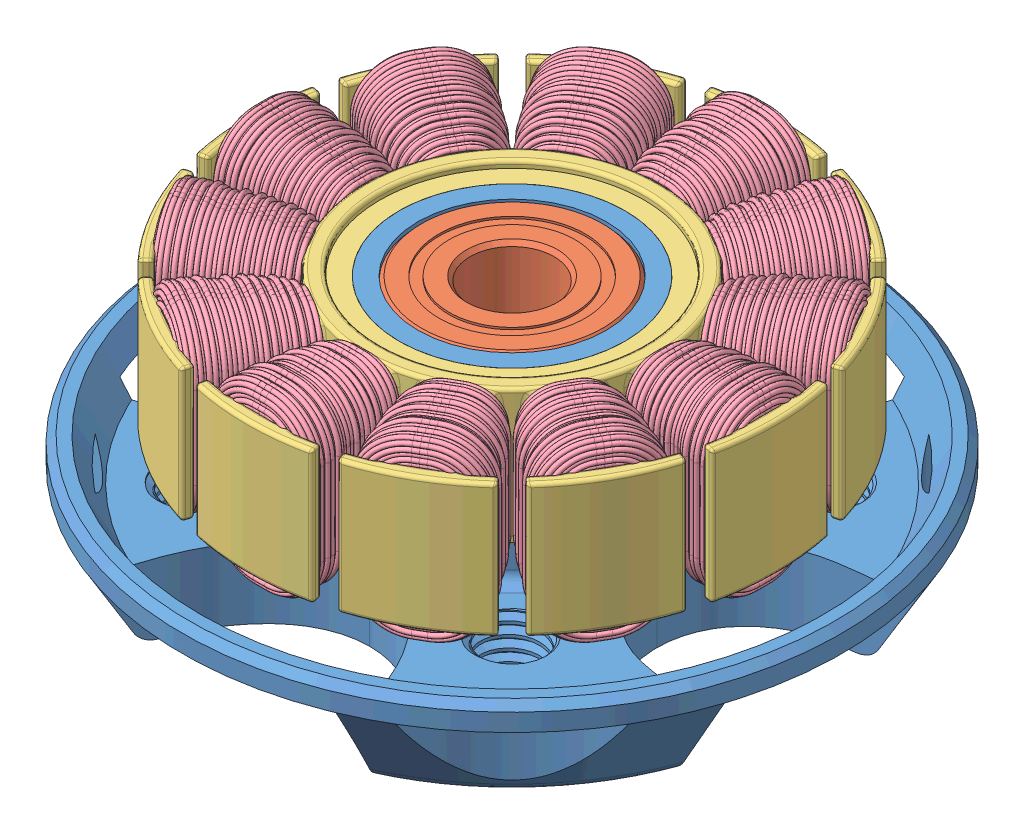
SolidWorks assembly STATOR RS2306, configuration Predeterminado. Lengths in mm.
Overall size (28 11.98 28).
16 component instances, 4 part files, 12 mates.
Components (placement in the parent):
- STATOR RS2306-1: STATOR RS2306 [Predeterminado] at origin size (28 10.77 28)
- BEARING-1: BEARING [Predeterminado] at (0 2.25 0) x (1 0 0) z (0 1 0) size (8 8 3.5)
- BEARING-2: BEARING [Predeterminado] at (0 8.85 0) x (-0.982082 0 -0.188455) z (0 -1 0) size (8 8 3.5)
- STATOR SLEEVE-1: STATOR SLEEVE [Predeterminado] at (0 5.25 0) size (22.5 5.67 22.5)
- WINDING-1: WINDING [Predeterminado] at (8.4112 8.075 0) size (4.68 7.47 4.47)
- WINDING-2: WINDING [Predeterminado] at (7.2843 8.075 4.2056) x (0.866025 0 0.5) z (-0.5 0 0.866025) size (4.68 7.47 4.47)
- WINDING-3: WINDING [Predeterminado] at (4.2056 8.075 7.2843) x (0.5 0 0.866025) z (-0.866025 0 0.5) size (4.68 7.47 4.47)
- WINDING-4: WINDING [Predeterminado] at (0 8.075 8.4112) x (0 0 1) z (-1 0 0) size (4.68 7.47 4.47)
- WINDING-5: WINDING [Predeterminado] at (-4.2056 8.075 7.2843) x (-0.5 0 0.866025) z (-0.866025 0 -0.5) size (4.68 7.47 4.47)
- WINDING-6: WINDING [Predeterminado] at (-7.2843 8.075 4.2056) x (-0.866025 0 0.5) z (-0.5 0 -0.866025) size (4.68 7.47 4.47)
- WINDING-7: WINDING [Predeterminado] at (-8.4112 8.075 0) x (-1 0 0) z (0 0 -1) size (4.68 7.47 4.47)
- WINDING-8: WINDING [Predeterminado] at (-7.2843 8.075 -4.2056) x (-0.866025 0 -0.5) z (0.5 0 -0.866025) size (4.68 7.47 4.47)
- WINDING-9: WINDING [Predeterminado] at (-4.2056 8.075 -7.2843) x (-0.5 0 -0.866025) z (0.866025 0 -0.5) size (4.68 7.47 4.47)
- WINDING-10: WINDING [Predeterminado] at (0 8.075 -8.4112) x (0 0 -1) z (1 0 0) size (4.68 7.47 4.47)
- WINDING-11: WINDING [Predeterminado] at (4.2056 8.075 -7.2843) x (0.5 0 -0.866025) z (0.866025 0 0.5) size (4.68 7.47 4.47)
- WINDING-12: WINDING [Predeterminado] at (7.2843 8.075 -4.2056) x (0.866025 0 -0.5) z (0.5 0 0.866025) size (4.68 7.47 4.47)
Mates (geometry in assembly coordinates):
- Coincidente1: coincident: plane of STATOR RS2306-1 through (0 0 0) normal (0 0 1); plane of assembly through (0 0 0) normal (0 0 1)
- Coincidente2: coincident: plane of STATOR RS2306-1 through (0 0 0) normal (0 1 0); plane of assembly through (0 0 0) normal (0 1 0)
- Coincidente3: coincident: plane of STATOR RS2306-1 through (0 0 0) normal (1 0 0); plane of assembly through (0 0 0) normal (1 0 0)
- Concéntrica1: concentric: cylinder of STATOR RS2306-1 through (0 0 0) axis (0 -1 0) radius 4; cylinder of BEARING-1 through (0 4 0) axis (0 1 0) radius 4.0005
- Coincidente4: coincident: plane of STATOR RS2306-1 through (-4 4 0) normal (0 -1 0); plane of BEARING-1 through (0 4 -3.8449) normal (0 1 0)
- Concéntrica2: concentric: cylinder of STATOR RS2306-1 through (0 0 0) axis (0 -1 0) radius 4; cylinder of BEARING-2 through (0 7.1 0) axis (0 -1 0) radius 4.0005
- Coincidente5: coincident: plane of STATOR RS2306-1 through (-3.5 7.1 0) normal (0 1 0); plane of BEARING-2 through (0.7246 7.1 -3.776) normal (0 -1 0)
- Concéntrica3: concentric: cylinder of STATOR RS2306-1 through (0 0 0) axis (0 -1 0) radius 4.8; cylinder of STATOR SLEEVE-1 through (0 10.6 0) axis (0 -1 0) radius 4.8
- Coincidente6: coincident: plane of STATOR RS2306-1 through (-4.95 5.25 0) normal (0 1 0); plane of STATOR SLEEVE-1 through (0 5.25 0) normal (0 -1 0)
- Coincidente7: coincident: plane of STATOR SLEEVE-1 through (0 5.25 0) normal (0 0 1); plane of assembly through (0 0 0) normal (0 0 1)
- Coincidente8: coincident: plane of STATOR SLEEVE-1 through (0 5.25 0) normal (0 0 1); plane of WINDING-1 through (8.4112 8.075 0) normal (0 0 1)
- Simétrico1: symmetric: plane of STATOR SLEEVE-1 through (6.2801 10.75 0.5) normal (0 1 0); plane of STATOR SLEEVE-1 through (6.2801 5.4 -0.5) normal (0 -1 0); plane of WINDING-1 through (8.4112 8.075 0) normal (0 1 0)
